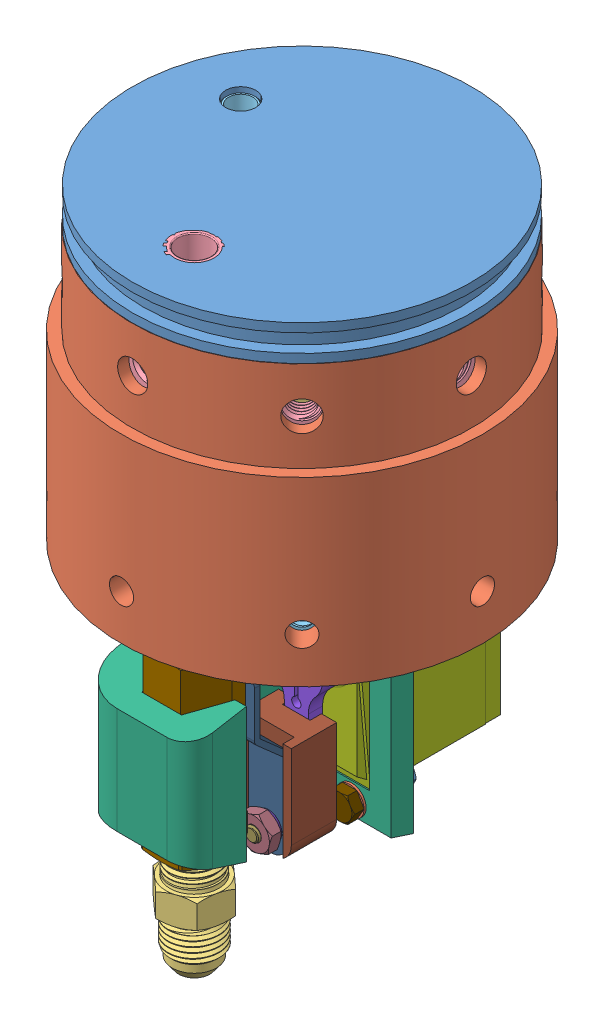
SolidWorks assembly Mojave Sphinx V1.2 Oxidizer Bulkhead Subassembly, configuration Default. Lengths in mm.
Overall size (120.19 175.01 101.4).
64 component instances, 30 part files, 37 mates.
Components (placement in the parent):
- BKHD-OX-O238–8NPT-4NPT Tank Bulkhead, Oxidizer, Mojave Sphinx-1: BKHD-OX-O238–8NPT-4NPT Tank Bulkhead, Oxidizer, Mojave Sphinx [Default] x (0 0 -1) z (-1 0 0) size (95 9.91 95)
- INRG-200S-8X3125C-8X250C Interface Ring, Tank, Mojave Sphinx-1: INRG-200S-8X3125C-8X250C Interface Ring, Tank, Mojave Sphinx [Default] at (0 -9.906 0) x (1 0 0) z (0 0 -1) size (101.35 76.2 101.35)
- Mojave Sphinx V1.2 Nut Retaining Ring Subassembly-1: Mojave Sphinx V1.2 Nut Retaining Ring Subassembly [Default] at (0 -9.906 0) x (-1 0 0) z (0 0 1) size (88.39 78.11 88.39)
  - NTRG-8X3125WN-8X25HN Nut Retaining Ring, Mojave Sphinx-1: NTRG-8X3125WN-8X25HN Nut Retaining Ring, Mojave Sphinx [Default] at origin size (88.39 78.11 88.39)
  - 94579A550_Steel Offset-Barrel Narrow-Base Weld Nut-1: 94579A550_Steel Offset-Barrel Narrow-Base Weld Nut [94579A550] at (0 18.9508 41.3942) x (0 -1 0) z (0 0 -1) size (25 15.88 6.02)
  - 95505A601_Medium-Strength Steel Hex Nut-1: 95505A601_Medium-Strength Steel Hex Nut [95505A601] at (0 63.5 40.8781) size (11.11 12.83 6.51)
  - 94579A550_Steel Offset-Barrel Narrow-Base Weld Nut-2: 94579A550_Steel Offset-Barrel Narrow-Base Weld Nut [94579A550] at (-29.2701 18.9508 29.2701) x (0 -1 0) z (0.707107 0 -0.707107) size (25 15.88 6.02)
  - 94579A550_Steel Offset-Barrel Narrow-Base Weld Nut-3: 94579A550_Steel Offset-Barrel Narrow-Base Weld Nut [94579A550] at (-41.3942 18.9508 0) x (0 -1 0) z (1 0 0) size (25 15.88 6.02)
  - 94579A550_Steel Offset-Barrel Narrow-Base Weld Nut-4: 94579A550_Steel Offset-Barrel Narrow-Base Weld Nut [94579A550] at (-29.2701 18.9508 -29.2701) x (0 -1 0) z (0.707107 0 0.707107) size (25 15.88 6.02)
  - 94579A550_Steel Offset-Barrel Narrow-Base Weld Nut-5: 94579A550_Steel Offset-Barrel Narrow-Base Weld Nut [94579A550] at (0 18.9508 -41.3942) x (0 -1 0) z (0 0 1) size (25 15.88 6.02)
  - 94579A550_Steel Offset-Barrel Narrow-Base Weld Nut-6: 94579A550_Steel Offset-Barrel Narrow-Base Weld Nut [94579A550] at (29.2701 18.9508 -29.2701) x (0 -1 0) z (-0.707107 0 0.707107) size (25 15.88 6.02)
  - 94579A550_Steel Offset-Barrel Narrow-Base Weld Nut-7: 94579A550_Steel Offset-Barrel Narrow-Base Weld Nut [94579A550] at (41.3942 18.9508 0) x (0 -1 0) z (-1 0 0) size (25 15.88 6.02)
  - 94579A550_Steel Offset-Barrel Narrow-Base Weld Nut-8: 94579A550_Steel Offset-Barrel Narrow-Base Weld Nut [94579A550] at (29.2701 18.9508 29.2701) x (0 -1 0) z (-0.707107 0 -0.707107) size (25 15.88 6.02)
  - 95505A601_Medium-Strength Steel Hex Nut-2: 95505A601_Medium-Strength Steel Hex Nut [95505A601] at (-28.9052 63.5 28.9052) x (0.707107 0 0.707107) z (-0.707107 0 0.707107) size (11.11 12.83 6.51)
  - 95505A601_Medium-Strength Steel Hex Nut-3: 95505A601_Medium-Strength Steel Hex Nut [95505A601] at (-40.8781 63.5 0) x (0 0 1) z (-1 0 0) size (11.11 12.83 6.51)
  - 95505A601_Medium-Strength Steel Hex Nut-4: 95505A601_Medium-Strength Steel Hex Nut [95505A601] at (-28.9052 63.5 -28.9052) x (-0.707107 0 0.707107) z (-0.707107 0 -0.707107) size (11.11 12.83 6.51)
  - 95505A601_Medium-Strength Steel Hex Nut-5: 95505A601_Medium-Strength Steel Hex Nut [95505A601] at (0 63.5 -40.8781) x (-1 0 0) z (0 0 -1) size (11.11 12.83 6.51)
  - 95505A601_Medium-Strength Steel Hex Nut-6: 95505A601_Medium-Strength Steel Hex Nut [95505A601] at (28.9052 63.5 -28.9052) x (-0.707107 0 -0.707107) z (0.707107 0 -0.707107) size (11.11 12.83 6.51)
  - 95505A601_Medium-Strength Steel Hex Nut-7: 95505A601_Medium-Strength Steel Hex Nut [95505A601] at (40.8781 63.5 0) x (0 0 -1) z (1 0 0) size (11.11 12.83 6.51)
  - 95505A601_Medium-Strength Steel Hex Nut-8: 95505A601_Medium-Strength Steel Hex Nut [95505A601] at (28.9052 63.5 28.9052) x (0.707107 0 -0.707107) z (0.707107 0 0.707107) size (11.11 12.83 6.51)
- SABV-04FF Servo Actuated Ball Valve Assembly, Mojave Sphinx-1: SABV-04FF Servo Actuated Ball Valve Assembly, Mojave Sphinx [Default] at (-18.936 -97.9629 45.6263) x (0 -1 0) z (0 0 1) size (61.96 34.92 92.62)
  - SABV-MNT-04V-3225S Mount, Servo Actuated Ball Valve, Hex Clearance, Mojave Sphinx-1: SABV-MNT-04V-3225S Mount, Servo Actuated Ball Valve, Hex Clearance, Mojave Sphinx [Default] at origin size (60.33 34.92 60.95)
  - DS3225 Servo 25kg-cm-1: DS3225 Servo 25kg-cm [Default] at (8.4201 28.8039 -92.6211) x (1 0 0) z (0 -1 0) size (54.41 46.01 19.94)
  - 25T Servo Horn-1: 25T Servo Horn [Default] at (17.9261 18.936 -48.0309) x (0 -1 0) z (1 0 0) size (14.73 6 34.84)
  - 4112T22_Compact High-Pressure Brass Ball Valve - Handle Removed-1: 4112T22_Compact High-Pressure Brass Ball Valve - Handle Removed [4112T22] at (-2.7129 18.936 -15.4511) x (0 1 0) z (-1 0 0) size (21.56 19.05 49.26)
  - 4112T22_Compact High-Pressure Brass Ball Valve - Handle ONLY-3: 4112T22_Compact High-Pressure Brass Ball Valve - Handle ONLY [4112T22] at (-2.7128 18.936 -15.4559) x (0 1 0) z (-1 0 0) size (15.12 15.24 48.28)
  - SABV-HCON-04V-3225S Handle Connector, Servo Actuated Ball Valve, Mojave Sphinx-1: SABV-HCON-04V-3225S Handle Connector, Servo Actuated Ball Valve, Mojave Sphinx [Default] at (29.3546 27.064 -34.5059) x (1 0 0) z (0 1 0) size (28.57 12.7 16.26)
  - 90272A194_ZINC-PLTD STL PAN HEAD PHILLIPS MACHINE SCREW-1: 90272A194_ZINC-PLTD STL PAN HEAD PHILLIPS MACHINE SCREW [90272A194] at (52.8496 18.936 -31.3309) x (-0.923728 -0.383049 0) z (0 0 -1) size (8.18 8.18 15.68)
  - 90480A009_LOW-STRENGTH STEEL HEX NUT-1: 90480A009_LOW-STRENGTH STEEL HEX NUT [90480A009] at (52.8496 18.936 -33.7189) x (0.950666 0.310215 0) z (-0.310215 0.950666 0) size (8.73 3.79 10.08)
  - 91290A115_BLACK-OXIDE CLASS 12.9 SOCKET HEAD CAP SCREW-1: 91290A115_BLACK-OXIDE CLASS 12.9 SOCKET HEAD CAP SCREW [91290A115] at (41.826 18.936 -50.7131) x (-0.923728 -0.383049 0) z (0 0 -1) size (5.5 5.5 13.21)
  - 98689A112_ METRIC GENERAL PURPOSE WASHERS-1: 98689A112_ METRIC GENERAL PURPOSE WASHERS [98689A112] at (41.826 18.936 -41.3131) size (6 6 0.6)
  - 92000A076_18-8 SS METRIC PAN HEAD PHIL MACHINE SCREW-1: 92000A076_18-8 SS METRIC PAN HEAD PHIL MACHINE SCREW [92000A076] at (17.9261 18.936 -48.4025) x (0.999336 -0.036448 0) z (0 0 1) size (6 6 5.52)
  - 92148A160_18-8 Stainless Steel Split Lock Washer-8: 92148A160_18-8 Stainless Steel Split Lock Washer [92148A160] at (52.8496 18.936 -36.2064) size (8.74 7.67 0.91)
  - 91280A044_MEDIUM-STRENGTH CLASS 8.8 STEEL HEX HEAD SCREW-1: 91280A044_MEDIUM-STRENGTH CLASS 8.8 STEEL HEX HEAD SCREW [91280A044] at (53.2996 23.9357 -60.5473) x (-1 0 0) z (0 0 1) size (7 8.08 19.18)
  - 90591A141_ZINC-PLATED STEEL HEX NUT-2: 90591A141_ZINC-PLATED STEEL HEX NUT [90591A141] at (53.2996 23.9357 -67.3085) x (-1 0 0) z (0 0 1) size (7 8.08 3.52)
  - 92148A160_18-8 Stainless Steel Split Lock Washer-3: 92148A160_18-8 Stainless Steel Split Lock Washer [92148A160] at (53.2996 23.936 -65.6985) size (8.74 7.67 0.91)
  - 98689A113_ METRIC GENERAL PURPOSE WASHERS-4: 98689A113_ METRIC GENERAL PURPOSE WASHERS [98689A113] at (53.2996 23.9357 -54.5973) size (8 8 0.6)
  - 98689A113_ METRIC GENERAL PURPOSE WASHERS-5: 98689A113_ METRIC GENERAL PURPOSE WASHERS [98689A113] at (53.2996 23.936 -64.7985) size (8 8 0.6)
  - 98689A113_ METRIC GENERAL PURPOSE WASHERS-9: 98689A113_ METRIC GENERAL PURPOSE WASHERS [98689A113] at (3.7995 23.9357 -54.5973) size (8 8 0.6)
  - 98689A113_ METRIC GENERAL PURPOSE WASHERS-10: 98689A113_ METRIC GENERAL PURPOSE WASHERS [98689A113] at (53.2996 13.9357 -54.5973) size (8 8 0.6)
  - 98689A113_ METRIC GENERAL PURPOSE WASHERS-11: 98689A113_ METRIC GENERAL PURPOSE WASHERS [98689A113] at (3.7995 13.9357 -54.5973) size (8 8 0.6)
  - 91280A044_MEDIUM-STRENGTH CLASS 8.8 STEEL HEX HEAD SCREW-2: 91280A044_MEDIUM-STRENGTH CLASS 8.8 STEEL HEX HEAD SCREW [91280A044] at (3.7995 23.9357 -60.5473) x (-1 0 0) z (0 0 1) size (7 8.08 19.18)
  - 91280A044_MEDIUM-STRENGTH CLASS 8.8 STEEL HEX HEAD SCREW-3: 91280A044_MEDIUM-STRENGTH CLASS 8.8 STEEL HEX HEAD SCREW [91280A044] at (53.2996 13.9357 -60.5473) x (-1 0 0) z (0 0 1) size (7 8.08 19.18)
  - 91280A044_MEDIUM-STRENGTH CLASS 8.8 STEEL HEX HEAD SCREW-4: 91280A044_MEDIUM-STRENGTH CLASS 8.8 STEEL HEX HEAD SCREW [91280A044] at (3.7995 13.9357 -60.5473) x (-1 0 0) z (0 0 1) size (7 8.08 19.18)
  - 90591A141_ZINC-PLATED STEEL HEX NUT-5: 90591A141_ZINC-PLATED STEEL HEX NUT [90591A141] at (3.7995 23.9357 -67.3085) x (-1 0 0) z (0 0 1) size (7 8.08 3.52)
  - 90591A141_ZINC-PLATED STEEL HEX NUT-6: 90591A141_ZINC-PLATED STEEL HEX NUT [90591A141] at (53.2996 13.9357 -67.3085) x (-1 0 0) z (0 0 1) size (7 8.08 3.52)
  - 90591A141_ZINC-PLATED STEEL HEX NUT-7: 90591A141_ZINC-PLATED STEEL HEX NUT [90591A141] at (3.7995 13.9357 -67.3085) x (-1 0 0) z (0 0 1) size (7 8.08 3.52)
  - 92148A160_18-8 Stainless Steel Split Lock Washer-5: 92148A160_18-8 Stainless Steel Split Lock Washer [92148A160] at (3.7995 23.936 -65.6985) size (8.74 7.67 0.91)
  - 92148A160_18-8 Stainless Steel Split Lock Washer-6: 92148A160_18-8 Stainless Steel Split Lock Washer [92148A160] at (53.2996 13.936 -65.6985) size (8.74 7.67 0.91)
  - 92148A160_18-8 Stainless Steel Split Lock Washer-7: 92148A160_18-8 Stainless Steel Split Lock Washer [92148A160] at (3.7995 13.936 -65.6985) size (8.74 7.67 0.91)
  - 98689A113_ METRIC GENERAL PURPOSE WASHERS-12: 98689A113_ METRIC GENERAL PURPOSE WASHERS [98689A113] at (3.7995 23.936 -64.7985) size (8 8 0.6)
  - 98689A113_ METRIC GENERAL PURPOSE WASHERS-13: 98689A113_ METRIC GENERAL PURPOSE WASHERS [98689A113] at (53.2996 13.936 -64.7985) size (8 8 0.6)
  - 98689A113_ METRIC GENERAL PURPOSE WASHERS-14: 98689A113_ METRIC GENERAL PURPOSE WASHERS [98689A113] at (3.7995 13.936 -64.7985) size (8 8 0.6)
- 50675K163_37 Degree Flared Fitting for Copper Tubing-1: 50675K163_37 Degree Flared Fitting for Copper Tubing [50675K163] at (0 -156.2735 30.1752) x (0 -1 0) z (0.979778 0 0.20009) size (36.71 18.33 15.88)
- 44665K137_Standard-Wall Aluminum Pipe Nipple-1: 44665K137_Standard-Wall Aluminum Pipe Nipple [44665K137] at (0 -50.8 30.1752) x (1 0 0) z (0 -1 0) size (14.4 14.28 102.75)
- 7768K21_Brass Threaded Check Valve-1: 7768K21_Brass Threaded Check Valve [7768K21] at (-29.3332 -14.732 -12.1502) x (1 0 0) z (0 -1 0) size (14.29 16.5 27.09)
- 50785K41_High-Pressure Brass Pipe Fitting-1: 50785K41_High-Pressure Brass Pipe Fitting [50785K41] at (-27.6136 -136.7525 -20.2863) x (0.519781 0.132808 -0.843914) z (-0.029136 0.990024 0.137856) size (14.24 19.84 15.04)
- 9396T31_High-Pressure Push-to-Connect Tube Fitting-1: 9396T31_High-Pressure Push-to-Connect Tube Fitting [9396T31] at (-29.3332 -31.115 -12.1502) x (1 0 0) z (0 -1 0) size (11.99 13.84 23.69)
- 9396T31_High-Pressure Push-to-Connect Tube Fitting-2: 9396T31_High-Pressure Push-to-Connect Tube Fitting [9396T31] at (-27.9577 -125.0593 -18.658) x (-0.853803 0.047066 -0.518465) z (-0.029136 0.990024 0.137856) size (11.99 13.84 23.69)
- 9685T3 QD Tube, 3.75in, Mojave Sphinx-1: 9685T3 QD Tube, 3.75in, Mojave Sphinx [Default] at (-27.9792 -124.3301 -18.5565) x (0.204723 0.140901 -0.968625) z (0.978386 0 0.206786) size (12.87 92.93 6.35)
- QDC-750X125FLG-281FB-8NPT Quick Disconnect, Female, Mojave Sphinx-1: QDC-750X125FLG-281FB-8NPT Quick Disconnect, Female, Mojave Sphinx [Default] at (-34.1196 -136.3939 -24.237) x (-0.853803 0.047066 -0.518465) z (0.502033 -0.189136 -0.843914) size (22.23 19.05 19.05)
- QDC-750x125FLG-270MB-O007-8NPT Quick Disconnect, Male, Mojave Sphinx-1: QDC-750x125FLG-270MB-O007-8NPT Quick Disconnect, Male, Mojave Sphinx [Default] at (-47.6737 -135.6467 -32.4676) x (-0.853803 0.047066 -0.518465) z (0.070208 0.997217 -0.02509) size (19.05 19.05 19.05)
- QDC-750X250CLP Quick Disconnect, Clip, Mojave Sphinx-1: QDC-750X250CLP Quick Disconnect, Clip, Mojave Sphinx [Default] at (-55.1084 -150.7691 -21.597) x (0.515841 -0.057822 -0.854731) z (0.853803 -0.047066 0.518465) size (24.13 25.4 12.7)
- 9452K15_Oil-Resistant Buna-N O-Ring-1: 9452K15_Oil-Resistant Buna-N O-Ring [9452K15] at (-50.1676 -135.5092 -33.982) x (0.070208 0.997217 -0.02509) z (0.853803 -0.047066 0.518465) size (7.24 7.24 1.78)
Mates (geometry in assembly coordinates):
- Coincident1: coincident aligned: plane of BKHD-OX-O238–8NPT-4NPT Tank Bulkhead, Oxidizer, Mojave Sphinx-1 through (0 -9.906 -47.498) normal (0 -1 0); circle of Mojave Sphinx V1.1 Interface Rings 2in Shoulder-1
- Concentric10: concentric anti-aligned: cylinder of BKHD-OX-O238–8NPT-4NPT Tank Bulkhead, Oxidizer, Mojave Sphinx-1 through (0 -6.35 30.1752) axis (0 -1 0) radius 5.5626; cylinder of SABV-04FF Servo Actuated Ball Valve Assembly, Mojave Sphinx-1/4112T22_Compact High-Pressure Brass Ball Valve - Handle Removed-1 through (0 -144.4893 30.1752) axis (0 1 0) radius 3.175
- Concentric25: concentric anti-aligned: cylinder of BKHD-OX-O238–8NPT-4NPT Tank Bulkhead, Oxidizer, Mojave Sphinx-1 through (0 -6.35 30.1752) axis (0 -1 0) radius 5.5626; cylinder of SABV-04FF Servo Actuated Ball Valve Assembly, Mojave Sphinx-1/4112T22_Compact High-Pressure Brass Ball Valve - Handle Removed-1 through (0 -144.4893 30.1752) axis (0 1 0) radius 3.175
- Concentric27: concentric anti-aligned: cylinder of BKHD-OX-O238–8NPT-4NPT Tank Bulkhead, Oxidizer, Mojave Sphinx-1 through (0 -6.35 30.1752) axis (0 -1 0) radius 5.5626; cylinder of 44665K137_Standard-Wall Aluminum Pipe Nipple (1)-1 through (0 0 30.1752) axis (0 1 0) radius 4.6228
- Distance4: distance = 6.35 mm anti-aligned: plane of 44665K137_Standard-Wall Aluminum Pipe Nipple (1)-1 through (0 0 34.798) normal (0 1 0); plane of BKHD-OX-O238–8NPT-4NPT Tank Bulkhead, Oxidizer, Mojave Sphinx-1 through (0 -6.35 -41.148) normal (0 -1 0)
- Concentric80: concentric aligned: cylinder of BKHD-OX-O238–8NPT-4NPT Tank Bulkhead, Oxidizer, Mojave Sphinx-1 through (-29.3332 -6.35 -12.1502) axis (0 -1 0) radius 4.2164; cylinder of 7768K21_Brass Threaded Check Valve-1 through (-29.3332 -1.27 -12.1502) axis (0 -1 0) radius 3.4163
- Distance16: distance = 5.08 mm anti-aligned: plane of 7768K21_Brass Threaded Check Valve-1 through (-29.3332 -1.27 -3.9013) normal (0 1 0); plane of BKHD-OX-O238–8NPT-4NPT Tank Bulkhead, Oxidizer, Mojave Sphinx-1 through (0 -6.35 -41.148) normal (0 -1 0)
- Coincident177: coincident anti-aligned: plane of BKHD-OX-O238–8NPT-4NPT Tank Bulkhead, Oxidizer, Mojave Sphinx-1 through (0 -9.906 -47.498) normal (0 -1 0); plane of Mojave Sphinx V1.2 Nut Retaining Ring Assem-1/NTRG-8X3125WN-8X25HN Nut Retaining Ring, Mojave Sphinx-1 through (0 -9.906 0) normal (0 1 0)
- Concentric208: concentric anti-aligned: cylinder of INRG-200S-8X3125C-8X250C Interface Ring, Tank, Mojave Sphinx-1 through (0 -87.7544 0) axis (0 -1 0) radius 44.45; cylinder of Mojave Sphinx V1.2 Nut Retaining Ring Assem-1/NTRG-8X3125WN-8X25HN Nut Retaining Ring, Mojave Sphinx-1 through (0 -86.106 0) axis (0 1 0) radius 41.656
- Distance5: distance = 6.35 mm anti-aligned: plane of Servo Valve Assem FF-1/4112T22_Compact High-Pressure Brass Ball Valve - Handle Removed-1 through (0 -95.25 30.1752) normal (0 1 0); plane of 44665K137_Standard-Wall Aluminum Pipe Nipple (1)-1 through (0 -101.6 34.798) normal (0 -1 0)
- Concentric312: concentric anti-aligned: cylinder of SABV-04FF Servo Actuated Ball Valve Assembly, Mojave Sphinx-1/4112T22_Compact High-Pressure Brass Ball Valve - Handle Removed-1 through (0 -144.4893 30.1752) axis (0 1 0) radius 3.175; cylinder of 50675K163_37 Degree Flared Fitting for Copper Tubing-1 through (0 -174.4345 30.1752) axis (0 -1 0) radius 3.7719
- Distance61: distance = 6.35 mm anti-aligned: plane of 50675K163_37 Degree Flared Fitting for Copper Tubing-1 through (0 -138.1125 30.1752) normal (0 1 0); plane of Servo Valve Assem FF-1/4112T22_Compact High-Pressure Brass Ball Valve - Handle Removed-1 through (0 -144.4625 40.9538) normal (0 -1 0)
- Concentric107: concentric anti-aligned: cylinder of 7768K21_Brass Threaded Check Valve-1 through (-29.3332 -1.27 -12.1502) axis (0 -1 0) radius 3.4163; cylinder of 9396T31_High-Pressure Push-to-Connect Tube Fitting (2)-1 through (-29.3332 -46.609 -12.1502) axis (0 1 0) radius 5.8547
- Distance21: distance = 5.08 mm anti-aligned: plane of 9396T31_High-Pressure Push-to-Connect Tube Fitting (2)-1 through (-29.3332 -23.114 -7.2558) normal (0 1 0); plane of 7768K21_Brass Threaded Check Valve-1 through (-29.3332 -28.194 -3.9013) normal (0 -1 0)
- Coincident257: coincident aligned: plane of 7768K21_Brass Threaded Check Valve-1 through (-29.3332 -14.732 -12.1502) normal (0 0 1); plane of 9396T31_High-Pressure Push-to-Connect Tube Fitting (2)-1 through (-29.3332 -31.115 -12.1502) normal (0 0 1)
- Concentric82: concentric anti-aligned: cylinder of 50785K41_High-Pressure Brass Pipe Fitting (3)-1 through (-38.4569 -136.1548 -26.8708) axis (-0.853803 0.047066 -0.518465) radius 3.2186; cylinder of QDC-750x125FLG-281FB-8NPT Quick Disconnect, Female, Mojave Sphinx-1 through (-34.1196 -136.3939 -24.237) axis (0.853803 -0.047066 0.518465) radius 6.731
- Concentric108: concentric aligned: cone of 50785K41_High-Pressure Brass Pipe Fitting (3)-1 through (-27.7246 -132.9805 -19.761) axis (0.029136 -0.990024 -0.137856); cylinder of 9396T31_High-Pressure Push-to-Connect Tube Fitting (2)-2 through (-28.4092 -109.7199 -16.5221) axis (0.029136 -0.990024 -0.137856) radius 3.4163
- Distance22: distance = 5.08 mm anti-aligned: plane of 9396T31_High-Pressure Push-to-Connect Tube Fitting (2)-2 through (-30.2686 -133.6305 -15.6306) normal (0.029136 -0.990024 -0.137856); plane of 50785K41_High-Pressure Brass Pipe Fitting (3)-1 through (-19.1504 -127.4067 -21.1273) normal (-0.029136 0.990024 0.137856)
- Coincident259: coincident anti-aligned: plane of 50785K41_High-Pressure Brass Pipe Fitting (3)-1 through (-27.6136 -136.7525 -20.2863) normal (0.519781 0.132808 -0.843914); plane of 9396T31_High-Pressure Push-to-Connect Tube Fitting (2)-2 through (-27.9577 -125.0593 -18.658) normal (-0.519781 -0.132808 0.843914)
- Concentric277: concentric aligned: cylinder of 9396T31_High-Pressure Push-to-Connect Tube Fitting (2)-1 through (-29.3332 -46.609 -12.1502) axis (0 1 0) radius 5.8547; cylinder of 9685T3 QD Tube, 3.75in, Mojave Sphinx-1 through (-29.3332 -46.5836 -12.1502) axis (0 1 0) radius 3.175
- Coincident235: coincident anti-aligned: plane of 9396T31_High-Pressure Push-to-Connect Tube Fitting (2)-1 through (-29.3332 -31.8516 -8.9752) normal (0 -1 0); plane of 9685T3 QD Tube, 3.75in, Mojave Sphinx-1 through (-29.3332 -31.8516 -12.1502) normal (0 1 0)
- Concentric278: concentric anti-aligned: cylinder of 9396T31_High-Pressure Push-to-Connect Tube Fitting (2)-2 through (-28.4092 -109.7199 -16.5221) axis (0.029136 -0.990024 -0.137856) radius 5.8547; cylinder of 9685T3 QD Tube, 3.75in, Mojave Sphinx-1 through (-27.9792 -124.3301 -18.5565) axis (-0.029136 0.990024 0.137856) radius 3.175
- Coincident261: coincident anti-aligned: plane of 9396T31_High-Pressure Push-to-Connect Tube Fitting (2)-2 through (-29.6295 -124.7517 -15.8771) normal (-0.029136 0.990024 0.137856); plane of 9685T3 QD Tube, 3.75in, Mojave Sphinx-1 through (-27.9792 -124.3301 -18.5565) normal (0.029136 -0.990024 -0.137856)
- Distance62: distance = 5.08 mm anti-aligned: plane of QDC-750x125FLG-281FB-8NPT Quick Disconnect, Female, Mojave Sphinx-1 through (-34.1196 -136.3939 -24.237) normal (0.853803 -0.047066 0.518465); plane of 50785K41_High-Pressure Brass Pipe Fitting (3)-1 through (-38.4569 -136.1548 -26.8708) normal (-0.853803 0.047066 -0.518465)
- Coincident263: coincident anti-aligned: plane of BKHD-OX-O238–8NPT-4NPT Tank Bulkhead, Oxidizer, Mojave Sphinx-1 through (0 0 0) normal (-1 0 0)
- Coincident264: coincident anti-aligned: plane of BKHD-OX-O238–8NPT-4NPT Tank Bulkhead, Oxidizer, Mojave Sphinx-1 through (0 0 0) normal (0 -1 0)
- Coincident265: coincident anti-aligned: plane of BKHD-OX-O238–8NPT-4NPT Tank Bulkhead, Oxidizer, Mojave Sphinx-1 through (0 0 0) normal (0 0 -1)
- Concentric313: concentric aligned: cylinder of BKHD-OX-O238–8NPT-4NPT Tank Bulkhead, Oxidizer, Mojave Sphinx-1 through (0 -48.1922 0) axis (0 -1 0) radius 47.498; cylinder of INRG-200S-8X3125C-8X250C Interface Ring, Tank, Mojave Sphinx-1 through (0 -87.7544 0) axis (0 -1 0) radius 47.625
- Coincident6: coincident aligned: plane of QDC-750x125FLG-270MB-O007-8NPT Quick Disconnect, Male, Mojave Sphinx-1 through (-47.6737 -135.6467 -32.4676) normal (-0.515841 0.057822 0.854731); plane of 9452K15_Oil-Resistant Buna-N O-Ring-1 through (-50.1676 -135.5092 -33.982) normal (-0.515841 0.057822 0.854731)
- Coincident7: coincident aligned: plane of QDC-750x125FLG-270MB-O007-8NPT Quick Disconnect, Male, Mojave Sphinx-1 through (-47.6737 -135.6467 -32.4676) normal (0.070208 0.997217 -0.02509); plane of 9452K15_Oil-Resistant Buna-N O-Ring-1 through (-50.1676 -135.5092 -33.982) normal (0.070208 0.997217 -0.02509)
- Concentric3: concentric anti-aligned: cylinder of QDC-750X125FLG-281FB-8NPT Quick Disconnect, Female, Mojave Sphinx-1 through (-53.0953 -135.3478 -35.7598) axis (-0.853803 0.047066 -0.518465) radius 3.5719; cylinder of QDC-750x125FLG-270MB-O007-8NPT Quick Disconnect, Male, Mojave Sphinx-1 through (-47.6737 -135.6467 -32.4676) axis (0.853803 -0.047066 0.518465) radius 1.1906
- Coincident8: coincident anti-aligned: plane of QDC-750X125FLG-281FB-8NPT Quick Disconnect, Female, Mojave Sphinx-1 through (-51.783 -126.0055 -37.0729) normal (-0.853803 0.047066 -0.518465); plane of QDC-750x125FLG-270MB-O007-8NPT Quick Disconnect, Male, Mojave Sphinx-1 through (-54.8723 -135.1486 -32.8154) normal (0.853803 -0.047066 0.518465)
- Width1: width anti-aligned: plane of QDC-750X250CLP Quick Disconnect, Clip, Mojave Sphinx-1 through (-53.1964 -145.0736 -42.9676) normal (0.853803 -0.047066 0.518465); plane of QDC-750X250CLP Quick Disconnect, Clip, Mojave Sphinx-1 through (-47.4495 -145.3904 -39.4778) normal (-0.853803 0.047066 -0.518465); plane of QDC-750x125FLG-270MB-O007-8NPT Quick Disconnect, Male, Mojave Sphinx-1 through (-60.7195 -134.6476 -29.2647) normal (-0.853803 0.047066 -0.518465); plane of QDC-750X125FLG-281FB-8NPT Quick Disconnect, Female, Mojave Sphinx-1 through (-49.4571 -128.8953 -35.0416) normal (0.853803 -0.047066 0.518465)
- Tangent6: tangent anti-aligned: cylinder of QDC-750X125FLG-281FB-8NPT Quick Disconnect, Female, Mojave Sphinx-1 through (-34.1196 -136.3939 -24.237) axis (0.853803 -0.047066 0.518465) radius 9.525; plane of QDC-750X250CLP Quick Disconnect, Clip, Mojave Sphinx-1 through (-54.6625 -144.4367 -21.7563) normal (0.070208 0.997217 -0.02509)
- Tangent7: tangent anti-aligned: cylinder of QDC-750X125FLG-281FB-8NPT Quick Disconnect, Female, Mojave Sphinx-1 through (-34.1196 -136.3939 -24.237) axis (0.853803 -0.047066 0.518465) radius 9.525; plane of QDC-750X250CLP Quick Disconnect, Clip, Mojave Sphinx-1 through (-44.769 -126.544 -42.181) normal (-0.517529 0.031219 0.855096)
- Parallel2: parallel anti-aligned: plane of QDC-750x125FLG-270MB-O007-8NPT Quick Disconnect, Male, Mojave Sphinx-1 through (-47.6737 -135.6467 -32.4676) normal (-0.515841 0.057822 0.854731); plane of QDC-750X250CLP Quick Disconnect, Clip, Mojave Sphinx-1 through (-55.1084 -150.7691 -21.597) normal (0.515841 -0.057822 -0.854731)
- Distance63: distance = 0.889 mm aligned: plane of 9452K15_Oil-Resistant Buna-N O-Ring-1 through (-50.1676 -135.5092 -33.982) normal (0.853803 -0.047066 0.518465); plane of QDC-750x125FLG-270MB-O007-8NPT Quick Disconnect, Male, Mojave Sphinx-1 through (-52.7037 -135.2682 -31.4985) normal (0.853803 -0.047066 0.518465)
